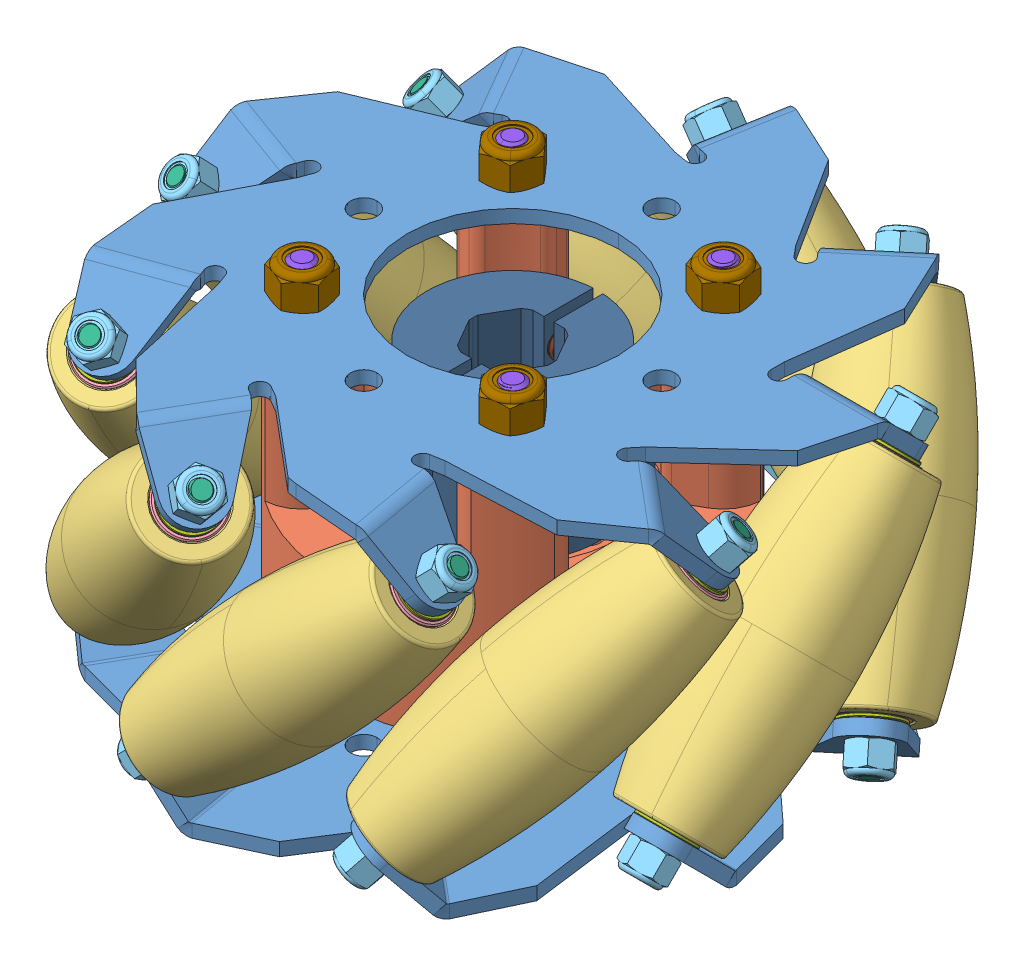
SolidWorks assembly Assem1, configuration Default. Lengths in mm.
Overall size (119.96 59.77 121.04).
89 component instances, 11 part files, 2 mates.
Components (placement in the parent):
- Mecanum Left Slant-1: Mecanum Left Slant [Default] at (53.1012 59.4979 77.2081) size (119.96 59.77 121.04)
  - Mecanum 2.STEP-1: Mecanum 2.STEP [Default] at origin size (119.96 59.77 121.04)
    - 3606-0000-0100 Side Plate.STEP-1: 3606-0000-0100 Side Plate.STEP [Default] at (-19.0769 -19.9696 22.3782) size (93.83 10.59 94.33)
    - 3606-0000-0100 Side Plate.STEP-2: 3606-0000-0100 Side Plate.STEP [Default] at (-19.0769 25.889 22.3782) x (1 0 0) z (0 0 -1) size (93.83 10.59 94.33)
    - 3606-XXXX-0100 Wheel Center.STEP-1: 3606-XXXX-0100 Wheel Center.STEP [Default] at (-19.0769 2.9597 22.3782) size (54 46 54)
    - 3606-XXXX-0100 Hi Durability Roller.STEP-1: 3606-XXXX-0100 Hi Durability Roller.STEP [Default] at (5.1459 -41.3984 63.1149) x (0.503693 -0.359647 0.78546) z (-0.696364 -0.707107 0.122788) size (28.35 23.77 47)
    - 3606-XXXX-0100 Roller Bearing.STEP-1: 3606-XXXX-0100 Roller Bearing.STEP [Default] at (-28.4431 -13.6618 64.9271) x (0.292157 -0.123026 0.948424) z (-0.655531 0.696322 0.292257) size (9 4 9)
    - 3606-XXXX-0100 Roller Locknut_90576A102.STEP-1: 3606-XXXX-0100 Roller Locknut_90576A102.STEP [Default] at (-30.184 -15.4296 65.2341) x (-0.521751 0.616262 0.589913) z (0.492801 -0.34673 0.798076) size (5.52 4.01 6.37)
    - 3606-XXXX-0100 Roller Axle.STEP-1: 3606-XXXX-0100 Roller Axle.STEP [Default] at (-12.0786 2.9552 62.0416) x (0.484544 -0.589424 -0.646372) z (0.529428 -0.390615 0.753078) size (4 60.01 4)
    - 3606-XXXX-0100 Roller Shim.STEP-1: 3606-XXXX-0100 Roller Shim.STEP [Default] at (-3.7599 24.6547 102.137) x (-0.324593 0.140076 0.935424) z (0.073634 -0.98223 0.172636) size (7.84 5.87 6.18)
    - 3606-XXXX-0100 Roller Bearing.STEP-2: 3606-XXXX-0100 Roller Bearing.STEP [Default] at (4.286 19.5722 59.1561) x (0.292157 -0.123026 0.948424) z (0.655531 -0.696322 -0.292257) size (9 4 9)
    - 3606-XXXX-0100 Roller Shim.STEP-2: 3606-XXXX-0100 Roller Shim.STEP [Default] at (35.261 37.7727 12.1321) x (-0.012231 -0.482096 -0.876033) z (-0.99905 0.042537 -0.00946) size (7.84 5.87 6.18)
    - 3606-XXXX-0100 Roller Locknut_90576A102.STEP-2: 3606-XXXX-0100 Roller Locknut_90576A102.STEP [Default] at (6.0269 21.34 58.8491) x (0.521751 -0.616262 -0.589913) z (0.492801 -0.34673 0.798076) size (5.52 4.01 6.37)
    - 3606-XXXX-0100 Roller Bearing.STEP-3: 3606-XXXX-0100 Roller Bearing.STEP [Default] at (-24.8203 19.5722 65.569) x (-0.38583 -0.123026 0.91433) z (0.690025 -0.696322 0.197486) size (9 4 9)
    - 3606-XXXX-0100 Roller Bearing.STEP-4: 3606-XXXX-0100 Roller Bearing.STEP [Default] at (-51.2391 19.5722 51.7725) x (-0.883283 -0.123026 0.45241) z (0.401649 -0.696322 0.594822) size (9 4 9)
    - 3606-XXXX-0100 Roller Bearing.STEP-5: 3606-XXXX-0100 Roller Bearing.STEP [Default] at (-62.6089 19.5722 24.2221) x (-0.967438 -0.123026 -0.221197) z (-0.074664 -0.696322 0.713835) size (9 4 9)
    - 3606-XXXX-0100 Roller Bearing.STEP-6: 3606-XXXX-0100 Roller Bearing.STEP [Default] at (-53.6095 19.5722 -4.1911) x (-0.598918 -0.123026 -0.791304) z (-0.51604 -0.696322 0.498837) size (9 4 9)
    - 3606-XXXX-0100 Roller Bearing.STEP-7: 3606-XXXX-0100 Roller Bearing.STEP [Default] at (-28.452 19.5722 -20.1723) x (0.049843 -0.123026 -0.991151) z (-0.715956 -0.696322 0.050427) size (9 4 9)
    - 3606-XXXX-0100 Roller Bearing.STEP-8: 3606-XXXX-0100 Roller Bearing.STEP [Default] at (1.0923 19.5722 -16.2436) x (0.675281 -0.123026 -0.727227) z (-0.580868 -0.696322 -0.421578) size (9 4 9)
    - 3606-XXXX-0100 Roller Bearing.STEP-9: 3606-XXXX-0100 Roller Bearing.STEP [Default] at (21.1992 19.5722 5.7567) x (0.984748 -0.123026 -0.123026) z (-0.173985 -0.696322 -0.696322) size (9 4 9)
    - 3606-XXXX-0100 Roller Bearing.STEP-10: 3606-XXXX-0100 Roller Bearing.STEP [Default] at (22.4605 19.5722 35.5343) x (0.833441 -0.123026 0.538741) z (0.314307 -0.696322 -0.645249) size (9 4 9)
    - 3606-XXXX-0100 Roller Shim.STEP-3: 3606-XXXX-0100 Roller Shim.STEP [Default] at (29.1344 37.7727 49.457) x (0.553733 -0.482096 -0.678942) z (-0.759236 0.042537 -0.649424) size (7.84 5.87 6.18)
    - 3606-XXXX-0100 Roller Shim.STEP-4: 3606-XXXX-0100 Roller Shim.STEP [Default] at (0.4492 37.7727 74.1114) x (0.8606 -0.482096 -0.164167) z (-0.164167 0.042537 -0.985515) size (7.84 5.87 6.18)
    - 3606-XXXX-0100 Roller Shim.STEP-5: 3606-XXXX-0100 Roller Shim.STEP [Default] at (-37.3725 37.7727 74.5592) x (0.764782 -0.482096 0.427424) z (0.507718 0.042537 -0.860473) size (7.84 5.87 6.18)
    - 3606-XXXX-0100 Roller Shim.STEP-6: 3606-XXXX-0100 Roller Shim.STEP [Default] at (-66.6334 37.7727 50.591) x (0.311114 -0.482096 0.819018) z (0.942036 0.042537 -0.332806) size (7.84 5.87 6.18)
    - 3606-XXXX-0100 Roller Shim.STEP-7: 3606-XXXX-0100 Roller Shim.STEP [Default] at (-73.6421 37.7727 13.4217) x (-0.288127 -0.482096 0.827385) z (0.935564 0.042537 0.350585) size (7.84 5.87 6.18)
    - 3606-XXXX-0100 Roller Shim.STEP-8: 3606-XXXX-0100 Roller Shim.STEP [Default] at (-55.1192 37.7727 -19.5568) x (-0.752551 -0.482096 0.448609) z (0.491332 0.042537 0.869933) size (7.84 5.87 6.18)
    - 3606-XXXX-0100 Roller Shim.STEP-9: 3606-XXXX-0100 Roller Shim.STEP [Default] at (-19.7316 37.7727 -32.9134) x (-0.864848 -0.482096 -0.140076) z (-0.1828 0.042537 0.98223) size (7.84 5.87 6.18)
    - 3606-XXXX-0100 Roller Shim.STEP-10: 3606-XXXX-0100 Roller Shim.STEP [Default] at (15.9623 37.7727 -20.3985) x (-0.572473 -0.482096 -0.663218) z (-0.771398 0.042537 0.63493) size (7.84 5.87 6.18)
    - 3606-XXXX-0100 Roller Locknut_90576A102.STEP-3: 3606-XXXX-0100 Roller Locknut_90576A102.STEP [Default] at (-23.2893 21.34 66.4529) x (0.778873 -0.616262 -0.116524) z (-0.135486 -0.34673 0.928128) size (5.52 4.01 6.37)
    - 3606-XXXX-0100 Roller Locknut_90576A102.STEP-4: 3606-XXXX-0100 Roller Locknut_90576A102.STEP [Default] at (-50.6345 21.34 53.4337) x (0.671552 -0.616262 0.411387) z (-0.700378 -0.34673 0.623899) size (5.52 4.01 6.37)
    - 3606-XXXX-0100 Roller Locknut_90576A102.STEP-5: 3606-XXXX-0100 Roller Locknut_90576A102.STEP [Default] at (-63.2135 21.34 25.8832) x (0.250004 -0.616262 0.746806) z (-0.937555 -0.34673 0.02774) size (5.52 4.01 6.37)
    - 3606-XXXX-0100 Roller Locknut_90576A102.STEP-6: 3606-XXXX-0100 Roller Locknut_90576A102.STEP [Default] at (-55.1405 21.34 -3.3072) x (-0.288524 -0.616262 0.732786) z (-0.73604 -0.34673 -0.581399) size (5.52 4.01 6.37)
    - 3606-XXXX-0100 Roller Locknut_90576A102.STEP-7: 3606-XXXX-0100 Roller Locknut_90576A102.STEP [Default] at (-30.1929 21.34 -20.4792) x (-0.692048 -0.616262 0.375887) z (-0.190123 -0.34673 -0.918494) size (5.52 4.01 6.37)
    - 3606-XXXX-0100 Roller Locknut_90576A102.STEP-8: 3606-XXXX-0100 Roller Locknut_90576A102.STEP [Default] at (-0.044 21.34 -17.5977) x (-0.771755 -0.616262 -0.156893) z (0.444754 -0.34673 -0.825816) size (5.52 4.01 6.37)
    - 3606-XXXX-0100 Roller Locknut_90576A102.STEP-9: 3606-XXXX-0100 Roller Locknut_90576A102.STEP [Default] at (21.1992 21.34 3.9889) x (-0.49035 -0.616262 -0.616262) z (0.871526 -0.34673 -0.34673) size (5.52 4.01 6.37)
    - 3606-XXXX-0100 Roller Locknut_90576A102.STEP-10: 3606-XXXX-0100 Roller Locknut_90576A102.STEP [Default] at (23.5968 21.34 34.1802) x (0.020496 -0.616262 -0.787275) z (0.890501 -0.34673 0.294596) size (5.52 4.01 6.37)
    - 3606-XXXX-0100 Roller Bearing.STEP-11: 3606-XXXX-0100 Roller Bearing.STEP [Default] at (-53.6018 -13.6618 48.952) x (-0.38583 -0.123026 0.91433) z (-0.690025 0.696322 -0.197486) size (9 4 9)
    - 3606-XXXX-0100 Roller Bearing.STEP-12: 3606-XXXX-0100 Roller Bearing.STEP [Default] at (-62.6058 -13.6618 20.5428) x (-0.883283 -0.123026 0.45241) z (-0.401649 0.696322 -0.594822) size (9 4 9)
    - 3606-XXXX-0100 Roller Bearing.STEP-13: 3606-XXXX-0100 Roller Bearing.STEP [Default] at (-51.2422 -13.6618 -7.0077) x (-0.967438 -0.123026 -0.221197) z (0.074664 0.696322 -0.713835) size (9 4 9)
    - 3606-XXXX-0100 Roller Bearing.STEP-14: 3606-XXXX-0100 Roller Bearing.STEP [Default] at (-24.828 -13.6618 -20.8081) x (-0.598918 -0.123026 -0.791304) z (0.51604 0.696322 -0.498837) size (9 4 9)
    - 3606-XXXX-0100 Roller Bearing.STEP-15: 3606-XXXX-0100 Roller Bearing.STEP [Default] at (4.2771 -13.6618 -14.4012) x (0.049843 -0.123026 -0.991151) z (0.715956 0.696322 -0.050427) size (9 4 9)
    - 3606-XXXX-0100 Roller Bearing.STEP-16: 3606-XXXX-0100 Roller Bearing.STEP [Default] at (22.4547 -13.6618 9.2152) x (0.675281 -0.123026 -0.727227) z (0.580868 0.696322 0.421578) size (9 4 9)
    - 3606-XXXX-0100 Roller Bearing.STEP-17: 3606-XXXX-0100 Roller Bearing.STEP [Default] at (21.1992 -13.6618 38.9907) x (0.984748 -0.123026 -0.123026) z (0.173985 0.696322 0.696322) size (9 4 9)
    - 3606-XXXX-0100 Roller Bearing.STEP-18: 3606-XXXX-0100 Roller Bearing.STEP [Default] at (1.0981 -13.6618 60.9931) x (0.833441 -0.123026 0.538741) z (-0.314307 0.696322 0.645249) size (9 4 9)
    - 3606-XXXX-0100 Roller Shim.STEP-11: 3606-XXXX-0100 Roller Shim.STEP [Default] at (-58.6113 24.6547 93.3225) x (-0.849932 0.140076 0.507932) z (-0.054562 -0.98223 0.179578) size (7.84 5.87 6.18)
    - 3606-XXXX-0100 Roller Shim.STEP-12: 3606-XXXX-0100 Roller Shim.STEP [Default] at (-94.9642 24.6547 51.3124) x (-0.977578 0.140076 -0.157227) z (-0.157227 -0.98223 0.102493) size (7.84 5.87 6.18)
    - 3606-XXXX-0100 Roller Shim.STEP-13: 3606-XXXX-0100 Roller Shim.STEP [Default] at (-95.8085 24.6547 -4.2363) x (-0.647805 0.140076 -0.748818) z (-0.186324 -0.98223 -0.022549) size (7.84 5.87 6.18)
    - 3606-XXXX-0100 Roller Shim.STEP-14: 3606-XXXX-0100 Roller Shim.STEP [Default] at (-60.7492 24.6547 -47.3318) x (-0.014916 0.140076 -0.990028) z (-0.128238 -0.98223 -0.137041) size (7.84 5.87 6.18)
    - 3606-XXXX-0100 Roller Shim.STEP-15: 3606-XXXX-0100 Roller Shim.STEP [Default] at (-6.191 24.6547 -57.8092) x (0.624951 0.140076 -0.767994) z (-0.010148 -0.98223 -0.187409) size (7.84 5.87 6.18)
    - 3606-XXXX-0100 Roller Shim.STEP-16: 3606-XXXX-0100 Roller Shim.STEP [Default] at (42.3378 24.6547 -30.7661) x (0.972397 0.140076 -0.186606) z (0.11269 -0.98223 -0.150086) size (7.84 5.87 6.18)
    - 3606-XXXX-0100 Roller Shim.STEP-17: 3606-XXXX-0100 Roller Shim.STEP [Default] at (62.13 24.6547 21.1439) x (0.864848 0.140076 0.482096) z (0.1828 -0.98223 -0.042537) size (7.84 5.87 6.18)
    - 3606-XXXX-0100 Roller Shim.STEP-18: 3606-XXXX-0100 Roller Shim.STEP [Default] at (43.9246 24.6547 73.6314) x (0.352626 0.140076 0.925221) z (0.167375 -0.98223 0.084916) size (7.84 5.87 6.18)
    - 3606-XXXX-0100 Roller Axle.STEP-2: 3606-XXXX-0100 Roller Axle.STEP [Default] at (-39.211 2.9552 57.2605) x (0.786662 -0.589424 -0.183691) z (-0.078503 -0.390615 0.917201) size (4 60.01 4)
    - 3606-XXXX-0100 Roller Axle.STEP-3: 3606-XXXX-0100 Roller Axle.STEP [Default] at (-56.9224 2.9552 36.1576) x (0.720693 -0.589424 0.364941) z (-0.649702 -0.390615 0.652156) size (4 60.01 4)
    - 3606-XXXX-0100 Roller Axle.STEP-4: 3606-XXXX-0100 Roller Axle.STEP [Default] at (-56.9255 2.9552 8.6072) x (0.317503 -0.589424 0.742813) z (-0.916899 -0.390615 0.08196) size (4 60.01 4)
    - 3606-XXXX-0100 Roller Axle.STEP-5: 3606-XXXX-0100 Roller Axle.STEP [Default] at (-39.2188 2.9552 -12.4996) x (-0.23425 -0.589424 0.773115) z (-0.755068 -0.390615 -0.526586) size (4 60.01 4)
    - 3606-XXXX-0100 Roller Axle.STEP-6: 3606-XXXX-0100 Roller Axle.STEP [Default] at (-12.0874 2.9552 -17.2867) x (-0.676394 -0.589424 0.441668) z (-0.239932 -0.390615 -0.888737) size (4 60.01 4)
    - 3606-XXXX-0100 Roller Axle.STEP-7: 3606-XXXX-0100 Roller Axle.STEP [Default] at (11.7735 2.9552 -3.5142) x (-0.802047 -0.589424 -0.096441) z (0.38747 -0.390615 -0.835037) size (4 60.01 4)
    - 3606-XXXX-0100 Roller Axle.STEP-8: 3606-XXXX-0100 Roller Axle.STEP [Default] at (21.1992 2.9552 22.3737) x (-0.552412 -0.589424 -0.589424) z (0.833571 -0.390615 -0.390615) size (4 60.01 4)
    - 3606-XXXX-0100 Roller Axle.STEP-9: 3606-XXXX-0100 Roller Axle.STEP [Default] at (11.7793 2.9552 48.2637) x (-0.044298 -0.589424 -0.806609) z (0.889635 -0.390615 0.236581) size (4 60.01 4)
    - 3606-XXXX-0100 Roller Locknut_90576A102.STEP-11: 3606-XXXX-0100 Roller Locknut_90576A102.STEP [Default] at (-55.1327 -15.4296 48.0682) x (-0.778873 0.616262 0.116524) z (-0.135486 -0.34673 0.928128) size (5.52 4.01 6.37)
    - 3606-XXXX-0100 Roller Locknut_90576A102.STEP-12: 3606-XXXX-0100 Roller Locknut_90576A102.STEP [Default] at (-63.2104 -15.4296 18.8816) x (-0.671552 0.616262 -0.411387) z (-0.700378 -0.34673 0.623899) size (5.52 4.01 6.37)
    - 3606-XXXX-0100 Roller Locknut_90576A102.STEP-13: 3606-XXXX-0100 Roller Locknut_90576A102.STEP [Default] at (-50.6375 -15.4296 -8.6688) x (-0.250004 0.616262 -0.746806) z (-0.937555 -0.34673 0.02774) size (5.52 4.01 6.37)
    - 3606-XXXX-0100 Roller Locknut_90576A102.STEP-14: 3606-XXXX-0100 Roller Locknut_90576A102.STEP [Default] at (-23.2971 -15.4296 -21.692) x (0.288524 0.616262 -0.732786) z (-0.73604 -0.34673 -0.581399) size (5.52 4.01 6.37)
    - 3606-XXXX-0100 Roller Locknut_90576A102.STEP-15: 3606-XXXX-0100 Roller Locknut_90576A102.STEP [Default] at (6.018 -15.4296 -14.0943) x (0.692048 0.616262 -0.375887) z (-0.190123 -0.34673 -0.918494) size (5.52 4.01 6.37)
    - 3606-XXXX-0100 Roller Locknut_90576A102.STEP-16: 3606-XXXX-0100 Roller Locknut_90576A102.STEP [Default] at (23.591 -15.4296 10.5694) x (0.771755 0.616262 0.156893) z (0.444754 -0.34673 -0.825816) size (5.52 4.01 6.37)
    - 3606-XXXX-0100 Roller Locknut_90576A102.STEP-17: 3606-XXXX-0100 Roller Locknut_90576A102.STEP [Default] at (21.1992 -15.4296 40.7585) x (0.49035 0.616262 0.616262) z (0.871526 -0.34673 -0.34673) size (5.52 4.01 6.37)
    - 3606-XXXX-0100 Roller Locknut_90576A102.STEP-18: 3606-XXXX-0100 Roller Locknut_90576A102.STEP [Default] at (-0.0382 -15.4296 62.3473) x (-0.020496 0.616262 0.787275) z (0.890501 -0.34673 0.294596) size (5.52 4.01 6.37)
    - 3606-XXXX-0100 Hi Durability Roller.STEP-2: 3606-XXXX-0100 Hi Durability Roller.STEP [Default] at (-26.7061 -41.3984 69.1544) x (-0.119033 -0.359647 0.925465) z (-0.612372 -0.707107 -0.353553) size (28.35 23.77 47)
    - 3606-XXXX-0100 Hi Durability Roller.STEP-3: 3606-XXXX-0100 Hi Durability Roller.STEP [Default] at (-54.9884 -41.3984 53.3069) x (-0.686062 -0.359647 0.632434) z (-0.241845 -0.707107 -0.664463) size (28.35 23.77 47)
    - 3606-XXXX-0100 Hi Durability Roller.STEP-4: 3606-XXXX-0100 Hi Durability Roller.STEP [Default] at (-66.4673 -41.3984 22.9874) x (-0.932075 -0.359647 0.043481) z (0.241845 -0.707107 -0.664463) size (28.35 23.77 47)
    - 3606-XXXX-0100 Hi Durability Roller.STEP-5: 3606-XXXX-0100 Hi Durability Roller.STEP [Default] at (-55.7716 -41.3984 -7.6171) x (-0.74196 -0.359647 -0.565818) z (0.612372 -0.707107 -0.353553) size (28.35 23.77 47)
    - 3606-XXXX-0100 Hi Durability Roller.STEP-6: 3606-XXXX-0100 Hi Durability Roller.STEP [Default] at (-27.9061 -41.3984 -24.1864) x (-0.204673 -0.359647 -0.910364) z (0.696364 -0.707107 0.122788) size (28.35 23.77 47)
    - 3606-XXXX-0100 Hi Durability Roller.STEP-7: 3606-XXXX-0100 Hi Durability Roller.STEP [Default] at (4.0907 -41.3984 -18.9677) x (0.428382 -0.359647 -0.828941) z (0.454519 -0.707107 0.541675) size (28.35 23.77 47)
    - 3606-XXXX-0100 Hi Durability Roller.STEP-8: 3606-XXXX-0100 Hi Durability Roller.STEP [Default] at (25.2472 -41.3984 5.5972) x (0.860993 -0.359647 -0.359647) z (0 -0.707107 0.707107) size (28.35 23.77 47)
    - 3606-XXXX-0100 Hi Durability Roller.STEP-9: 3606-XXXX-0100 Hi Durability Roller.STEP [Default] at (25.6639 -41.3984 38.0142) x (0.890735 -0.359647 0.27793) z (-0.454519 -0.707107 0.541675) size (28.35 23.77 47)
    - 2800-0004-0055_90128A207.STEP-1: 2800-0004-0055_90128A207.STEP [Default] at (-35.0769 32.9597 38.3782) x (0.999526 0 0.030777) z (0 1 0) size (9.08 9.66 59.77)
    - 2800-0004-0055_90128A207.STEP-2: 2800-0004-0055_90128A207.STEP [Default] at (-35.0769 32.9597 6.3782) x (-0.030777 0 0.999526) z (0 1 0) size (9.08 9.66 59.77)
    - 2800-0004-0055_90128A207.STEP-3: 2800-0004-0055_90128A207.STEP [Default] at (-3.0769 32.9597 6.3782) x (-0.999526 0 -0.030777) z (0 1 0) size (9.08 9.66 59.77)
    - 2800-0004-0055_90128A207.STEP-4: 2800-0004-0055_90128A207.STEP [Default] at (-3.0769 32.9597 38.3782) x (0.030777 0 -0.999526) z (0 1 0) size (9.08 9.66 59.77)
    - 2812-0004-0007_90576A103.STEP-1: 2812-0004-0007_90576A103.STEP [Default] at (-35.0769 27.9597 38.3782) x (0.654056 0 0.756446) z (-0.756446 0 0.654056) size (7.02 4.86 8.1)
    - 2812-0004-0007_90576A103.STEP-2: 2812-0004-0007_90576A103.STEP [Default] at (-35.0769 27.9597 6.3782) x (-0.756446 0 0.654056) z (-0.654056 0 -0.756446) size (7.02 4.86 8.1)
    - 2812-0004-0007_90576A103.STEP-3: 2812-0004-0007_90576A103.STEP [Default] at (-3.0769 27.9597 6.3782) x (-0.654056 0 -0.756446) z (0.756446 0 -0.654056) size (7.02 4.86 8.1)
    - 2812-0004-0007_90576A103.STEP-4: 2812-0004-0007_90576A103.STEP [Default] at (-3.0769 27.9597 38.3782) x (0.756446 0 -0.654056) z (0.654056 0 0.756446) size (7.02 4.86 8.1)
- 12mm Hyper Hub.STEP-1: 12mm Hyper Hub.STEP [Default] at (26.2861 53.0574 117.7049) x (0.999999 0 -0.001105) z (0 1 0) size (26 26 21)
  - 1310-0016-4012.STEP-1: 1310-0016-4012.STEP [Default] at (7.7672 18.1012 8.4002) size (26 26 21)
  - 2800-0004-0014_90128A207.STEP-1: 2800-0004-0014_90128A207.STEP [Default] at (-1.9828 25.8512 24.0002) x (0 0 1) z (-1 0 0) size (7 7 18.01)
  - 2800-0004-0014_90128A207.STEP-2: 2800-0004-0014_90128A207.STEP [Default] at (17.5172 10.3512 24.0002) x (0 0 1) z (1 0 0) size (7 7 18.01)
Mates (geometry in assembly coordinates):
- Concentric4: concentric: circle of Mecanum Left Slant-1/Mecanum 2.STEP-1/3606-XXXX-0100 Wheel Center.STEP-1; circle of 12mm Hyper Hub.STEP-1/1310-0016-4012.STEP-1
- Tangent1: tangent: circle of Mecanum Left Slant-1/Mecanum 2.STEP-1/3606-XXXX-0100 Wheel Center.STEP-1; circle of 12mm Hyper Hub.STEP-1/1310-0016-4012.STEP-1
